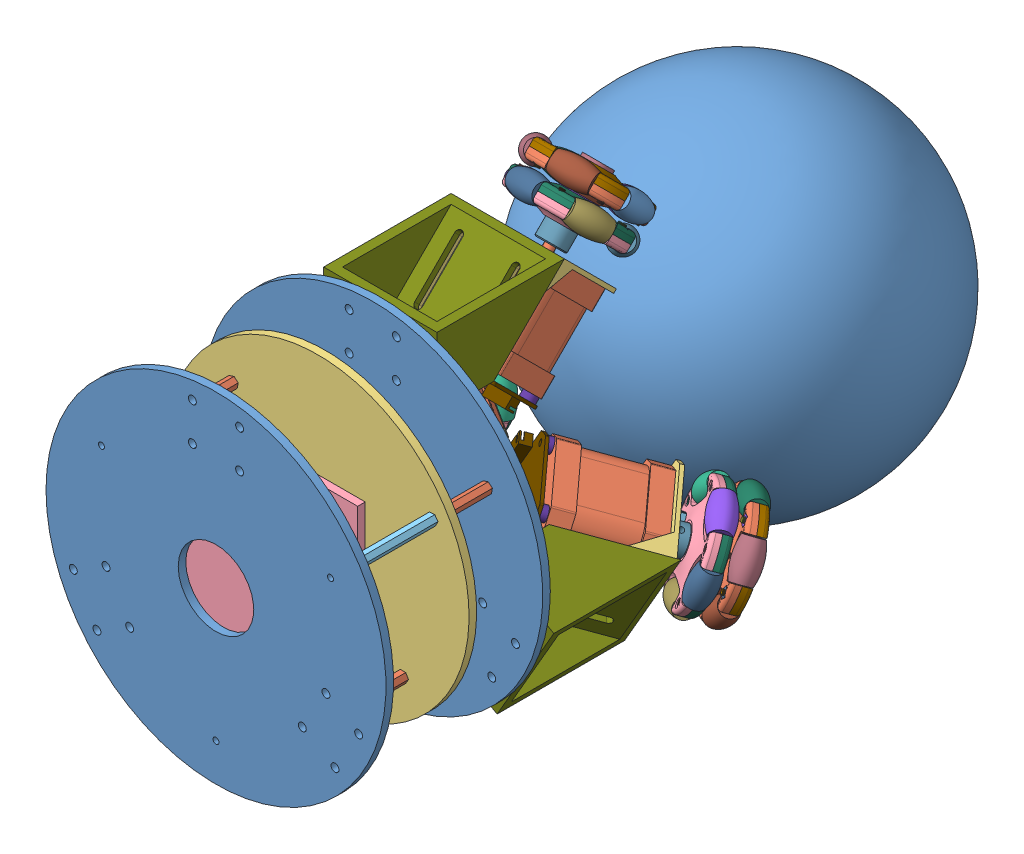
SolidWorks assembly 轮球平衡机器人, configuration 默认. Lengths in mm.
Overall size (282.14 310.32 417.32).
195 component instances, 61 part files, 35 mates.
Components (placement in the parent):
- 底盘底层-1: 底盘底层 [默认] at (0 81.589 0) size (180 180 4)
- 轮电机装配-1: 轮电机装配 [默认] at (-247.6697 -4.8466 -119.7715) x (0.62563 0.330076 -0.70685) z (-0.483308 0.875243 -0.019064) size (112.27 117.96 63.25)
  - 42步进电机-1: 42步进电机 [Default] at (113.7797 -206.2562 -45.9286) x (-0.026961 0 0.999636) z (0 1 0) size (42 47 67.8)
  - 42步进电机连接件-1: 42步进电机连接件 [默认] at (113.7797 -156.4562 -45.9286) x (0.026961 0 -0.999636) z (-0.999636 0 -0.026961) size (50 53 51)
  - 58mm全向轮-2: 58mm全向轮 [默认] at (113.7797 -145.9562 -45.9286) size (67.49 41.74 62.32)
    - 58MMQUANXIANGLUN_DAN-1: 58MMQUANXIANGLUN_DAN [默认] at origin size (67.49 27.49 60.7)
      - DANGPIAN-1-1: DANGPIAN-1 [默认] at origin size (55.41 8.9 53.54)
      - GUNZHOU-1-1: GUNZHOU-1 [默认] at origin size (10.16 3.8 24.74)
      - GUNZI-1-1: GUNZI-1 [默认] at origin size (19.85 20.87 20.84)
      - GUNZHOU_1-1-1: GUNZHOU_1-1 [默认] at origin size (25.2 3.8 3.8)
      - GUNZI_1-1-1: GUNZI_1-1 [默认] at origin size (19.2 13.87 13.87)
      - GUNZHOU_2-1-1: GUNZHOU_2-1 [默认] at origin size (10.16 3.8 24.74)
      - GUNZI_2-1-1: GUNZI_2-1 [默认] at origin size (19.85 20.87 20.84)
      - GUNZHOU_3-1-1: GUNZHOU_3-1 [默认] at origin size (21.86 3.8 16.83)
      - GUNZI_3-1-1: GUNZI_3-1 [默认] at origin size (20.83 27.49 22.24)
      - GUNZHOU_4-1-1: GUNZHOU_4-1 [默认] at origin size (21.86 3.8 16.83)
      - GUNZI_4-1-1: GUNZI_4-1 [默认] at origin size (20.83 27.49 22.24)
      - DANGPIAN_HOU-1-1: DANGPIAN_HOU-1 [默认] at origin size (55.39 8.9 53.54)
      - M3X8-1-1: M3X8-1 [默认] at origin size (4.21 9.65 4.2)
      - M3LUOMU-1-1: M3LUOMU-1 [默认] at origin size (4.9 2 5.66)
      - M3X8_1-1-1: M3X8_1-1 [默认] at origin size (4.2 9.65 4.2)
      - M3LUOMU_1-1-1: M3LUOMU_1-1 [默认] at origin size (5.38 2 5.53)
      - M3X8_2-1-1: M3X8_2-1 [默认] at origin size (4.2 9.65 4.2)
      - M3LUOMU_2-1-1: M3LUOMU_2-1 [默认] at origin size (5.63 2 5.17)
      - M3X8_3-1-1: M3X8_3-1 [默认] at origin size (4.2 9.65 4.2)
      - M3LUOMU_3-1-1: M3LUOMU_3-1 [默认] at origin size (5.63 2 5.17)
      - M3X8_4-1-1: M3X8_4-1 [默认] at origin size (4.2 9.65 4.2)
      - M3LUOMU_4-1-1: M3LUOMU_4-1 [默认] at origin size (5.38 2 5.53)
    - LIANJIEQUAN-1-1: LIANJIEQUAN-1 [默认] at origin size (17 2.5 17)
    - 58MMQUANXIANGLUN_DAN_1-1: 58MMQUANXIANGLUN_DAN_1 [默认] at origin size (67.49 27.49 60.7)
      - DANGPIAN-3-1: DANGPIAN-3 [默认] at origin size (55.41 8.9 53.54)
      - GUNZHOU-3-1: GUNZHOU-3 [默认] at origin size (10.16 3.8 24.74)
      - GUNZI-3-1: GUNZI-3 [默认] at origin size (19.85 20.87 20.84)
      - GUNZHOU_1-3-1: GUNZHOU_1-3 [默认] at origin size (21.86 3.8 16.83)
      - GUNZI_1-3-1: GUNZI_1-3 [默认] at origin size (20.83 27.49 22.24)
      - GUNZHOU_2-3-1: GUNZHOU_2-3 [默认] at origin size (21.86 3.8 16.83)
      - GUNZI_2-3-1: GUNZI_2-3 [默认] at origin size (20.83 27.49 22.24)
      - GUNZHOU_3-3-1: GUNZHOU_3-3 [默认] at origin size (10.16 3.8 24.74)
      - GUNZI_3-3-1: GUNZI_3-3 [默认] at origin size (19.85 20.87 20.84)
      - GUNZHOU_4-3-1: GUNZHOU_4-3 [默认] at origin size (25.2 3.8 3.8)
      - GUNZI_4-3-1: GUNZI_4-3 [默认] at origin size (19.2 13.87 13.87)
      - DANGPIAN_HOU-3-1: DANGPIAN_HOU-3 [默认] at origin size (55.39 8.9 53.54)
      - M3X8-3-1: M3X8-3 [默认] at origin size (4.2 9.65 4.2)
      - M3LUOMU-3-1: M3LUOMU-3 [默认] at origin size (5.63 2 5.17)
      - M3X8_1-3-1: M3X8_1-3 [默认] at origin size (4.2 9.65 4.2)
      - M3LUOMU_1-3-1: M3LUOMU_1-3 [默认] at origin size (5.38 2 5.53)
      - M3X8_2-3-1: M3X8_2-3 [默认] at origin size (4.21 9.65 4.2)
      - M3LUOMU_2-3-1: M3LUOMU_2-3 [默认] at origin size (4.9 2 5.66)
      - M3X8_3-3-1: M3X8_3-3 [默认] at origin size (4.2 9.65 4.2)
      - M3LUOMU_3-3-1: M3LUOMU_3-3 [默认] at origin size (5.38 2 5.53)
      - M3X8_4-3-1: M3X8_4-3 [默认] at origin size (4.2 9.65 4.2)
      - M3LUOMU_4-3-1: M3LUOMU_4-3 [默认] at origin size (5.63 2 5.17)
    - 20170615_LIANZHOUQITAOJIAN4X23-1-1: 20170615_LIANZHOUQITAOJIAN4X23-1 [默认] at origin size (13.9 6 13.9)
    - 20170615_LIANZHOUQI_4X23-1-1: 20170615_LIANZHOUQI_4X23-1 [默认] at origin size (13.9 23 13.9)
    - M4X12-1-1: M4X12-1 [默认] at origin size (6.9 15.15 7.04)
  - 底盘连接件-1: 底盘连接件 [默认] at (84.5995 -209.4562 -76.7265) x (-0.026961 0 0.999636) z (0.70685 -0.707107 0.019064) size (60 67.48 37.48)
  - 3mm尼龙垫圈高度3mm-1: 3mm尼龙垫圈高度3mm [默认] at (129.692 -209.2562 -61.0051) size (7 3 7)
  - 3mm尼龙垫圈高度3mm-2: 3mm尼龙垫圈高度3mm [默认] at (128.8562 -209.2562 -30.0163) size (7 3 7)
  - 3mm尼龙垫圈高度3mm-3: 3mm尼龙垫圈高度3mm [默认] at (98.7033 -209.2562 -61.8408) size (7 3 7)
  - 3mm尼龙垫圈高度3mm-4: 3mm尼龙垫圈高度3mm [默认] at (97.8675 -209.2562 -30.8521) size (7 3 7)
  - 42闭环PCB-1: 42闭环PCB [默认] at (98.7033 -209.2562 -61.8408) x (-1 0 0) z (0 -1 0) size (46.56 42.8 7)
- 轮电机装配-4: 轮电机装配 [默认] at (48.9795 339.2949 -119.7715) x (-0.026961 -0.70685 -0.70685) z (0.999636 -0.019064 -0.019064) size (112.27 117.96 63.25)
  - 42步进电机-1: 42步进电机 [Default] at (113.7797 -206.2562 -45.9286) x (-0.026961 0 0.999636) z (0 1 0) size (42 47 67.8)
  - 42步进电机连接件-1: 42步进电机连接件 [默认] at (113.7797 -156.4562 -45.9286) x (0.026961 0 -0.999636) z (-0.999636 0 -0.026961) size (50 53 51)
  - 58mm全向轮-2: 58mm全向轮 [默认] at (113.7797 -145.9562 -45.9286) size (67.49 41.74 62.32)
    - 58MMQUANXIANGLUN_DAN-1: 58MMQUANXIANGLUN_DAN [默认] at origin size (67.49 27.49 60.7)
      - DANGPIAN-1-1: DANGPIAN-1 [默认] at origin size (55.41 8.9 53.54)
      - GUNZHOU-1-1: GUNZHOU-1 [默认] at origin size (10.16 3.8 24.74)
      - GUNZI-1-1: GUNZI-1 [默认] at origin size (19.85 20.87 20.84)
      - GUNZHOU_1-1-1: GUNZHOU_1-1 [默认] at origin size (25.2 3.8 3.8)
      - GUNZI_1-1-1: GUNZI_1-1 [默认] at origin size (19.2 13.87 13.87)
      - GUNZHOU_2-1-1: GUNZHOU_2-1 [默认] at origin size (10.16 3.8 24.74)
      - GUNZI_2-1-1: GUNZI_2-1 [默认] at origin size (19.85 20.87 20.84)
      - GUNZHOU_3-1-1: GUNZHOU_3-1 [默认] at origin size (21.86 3.8 16.83)
      - GUNZI_3-1-1: GUNZI_3-1 [默认] at origin size (20.83 27.49 22.24)
      - GUNZHOU_4-1-1: GUNZHOU_4-1 [默认] at origin size (21.86 3.8 16.83)
      - GUNZI_4-1-1: GUNZI_4-1 [默认] at origin size (20.83 27.49 22.24)
      - DANGPIAN_HOU-1-1: DANGPIAN_HOU-1 [默认] at origin size (55.39 8.9 53.54)
      - M3X8-1-1: M3X8-1 [默认] at origin size (4.21 9.65 4.2)
      - M3LUOMU-1-1: M3LUOMU-1 [默认] at origin size (4.9 2 5.66)
      - M3X8_1-1-1: M3X8_1-1 [默认] at origin size (4.2 9.65 4.2)
      - M3LUOMU_1-1-1: M3LUOMU_1-1 [默认] at origin size (5.38 2 5.53)
      - M3X8_2-1-1: M3X8_2-1 [默认] at origin size (4.2 9.65 4.2)
      - M3LUOMU_2-1-1: M3LUOMU_2-1 [默认] at origin size (5.63 2 5.17)
      - M3X8_3-1-1: M3X8_3-1 [默认] at origin size (4.2 9.65 4.2)
      - M3LUOMU_3-1-1: M3LUOMU_3-1 [默认] at origin size (5.63 2 5.17)
      - M3X8_4-1-1: M3X8_4-1 [默认] at origin size (4.2 9.65 4.2)
      - M3LUOMU_4-1-1: M3LUOMU_4-1 [默认] at origin size (5.38 2 5.53)
    - LIANJIEQUAN-1-1: LIANJIEQUAN-1 [默认] at origin size (17 2.5 17)
    - 58MMQUANXIANGLUN_DAN_1-1: 58MMQUANXIANGLUN_DAN_1 [默认] at origin size (67.49 27.49 60.7)
      - DANGPIAN-3-1: DANGPIAN-3 [默认] at origin size (55.41 8.9 53.54)
      - GUNZHOU-3-1: GUNZHOU-3 [默认] at origin size (10.16 3.8 24.74)
      - GUNZI-3-1: GUNZI-3 [默认] at origin size (19.85 20.87 20.84)
      - GUNZHOU_1-3-1: GUNZHOU_1-3 [默认] at origin size (21.86 3.8 16.83)
      - GUNZI_1-3-1: GUNZI_1-3 [默认] at origin size (20.83 27.49 22.24)
      - GUNZHOU_2-3-1: GUNZHOU_2-3 [默认] at origin size (21.86 3.8 16.83)
      - GUNZI_2-3-1: GUNZI_2-3 [默认] at origin size (20.83 27.49 22.24)
      - GUNZHOU_3-3-1: GUNZHOU_3-3 [默认] at origin size (10.16 3.8 24.74)
      - GUNZI_3-3-1: GUNZI_3-3 [默认] at origin size (19.85 20.87 20.84)
      - GUNZHOU_4-3-1: GUNZHOU_4-3 [默认] at origin size (25.2 3.8 3.8)
      - GUNZI_4-3-1: GUNZI_4-3 [默认] at origin size (19.2 13.87 13.87)
      - DANGPIAN_HOU-3-1: DANGPIAN_HOU-3 [默认] at origin size (55.39 8.9 53.54)
      - M3X8-3-1: M3X8-3 [默认] at origin size (4.2 9.65 4.2)
      - M3LUOMU-3-1: M3LUOMU-3 [默认] at origin size (5.63 2 5.17)
      - M3X8_1-3-1: M3X8_1-3 [默认] at origin size (4.2 9.65 4.2)
      - M3LUOMU_1-3-1: M3LUOMU_1-3 [默认] at origin size (5.38 2 5.53)
      - M3X8_2-3-1: M3X8_2-3 [默认] at origin size (4.21 9.65 4.2)
      - M3LUOMU_2-3-1: M3LUOMU_2-3 [默认] at origin size (4.9 2 5.66)
      - M3X8_3-3-1: M3X8_3-3 [默认] at origin size (4.2 9.65 4.2)
      - M3LUOMU_3-3-1: M3LUOMU_3-3 [默认] at origin size (5.38 2 5.53)
      - M3X8_4-3-1: M3X8_4-3 [默认] at origin size (4.2 9.65 4.2)
      - M3LUOMU_4-3-1: M3LUOMU_4-3 [默认] at origin size (5.63 2 5.17)
    - 20170615_LIANZHOUQITAOJIAN4X23-1-1: 20170615_LIANZHOUQITAOJIAN4X23-1 [默认] at origin size (13.9 6 13.9)
    - 20170615_LIANZHOUQI_4X23-1-1: 20170615_LIANZHOUQI_4X23-1 [默认] at origin size (13.9 23 13.9)
    - M4X12-1-1: M4X12-1 [默认] at origin size (6.9 15.15 7.04)
  - 底盘连接件-1: 底盘连接件 [默认] at (84.5995 -209.4562 -76.7265) x (-0.026961 0 0.999636) z (0.70685 -0.707107 0.019064) size (60 67.48 37.48)
  - 3mm尼龙垫圈高度3mm-1: 3mm尼龙垫圈高度3mm [默认] at (129.692 -209.2562 -61.0051) size (7 3 7)
  - 3mm尼龙垫圈高度3mm-2: 3mm尼龙垫圈高度3mm [默认] at (128.8562 -209.2562 -30.0163) size (7 3 7)
  - 3mm尼龙垫圈高度3mm-3: 3mm尼龙垫圈高度3mm [默认] at (98.7033 -209.2562 -61.8408) size (7 3 7)
  - 3mm尼龙垫圈高度3mm-4: 3mm尼龙垫圈高度3mm [默认] at (97.8675 -209.2562 -30.8521) size (7 3 7)
  - 42闭环PCB-1: 42闭环PCB [默认] at (98.7033 -209.2562 -61.8408) x (-1 0 0) z (0 -1 0) size (46.56 42.8 7)
- 轮电机装配-5: 轮电机装配 [默认] at (198.6902 -89.6815 -119.7715) x (-0.598669 0.376774 -0.70685) z (-0.516328 -0.856179 -0.019064) size (112.27 117.96 63.25)
  - 42步进电机-1: 42步进电机 [Default] at (113.7797 -206.2562 -45.9286) x (-0.026961 0 0.999636) z (0 1 0) size (42 47 67.8)
  - 42步进电机连接件-1: 42步进电机连接件 [默认] at (113.7797 -156.4562 -45.9286) x (0.026961 0 -0.999636) z (-0.999636 0 -0.026961) size (50 53 51)
  - 58mm全向轮-2: 58mm全向轮 [默认] at (113.7797 -145.9562 -45.9286) size (67.49 41.74 62.32)
    - 58MMQUANXIANGLUN_DAN-1: 58MMQUANXIANGLUN_DAN [默认] at origin size (67.49 27.49 60.7)
      - DANGPIAN-1-1: DANGPIAN-1 [默认] at origin size (55.41 8.9 53.54)
      - GUNZHOU-1-1: GUNZHOU-1 [默认] at origin size (10.16 3.8 24.74)
      - GUNZI-1-1: GUNZI-1 [默认] at origin size (19.85 20.87 20.84)
      - GUNZHOU_1-1-1: GUNZHOU_1-1 [默认] at origin size (25.2 3.8 3.8)
      - GUNZI_1-1-1: GUNZI_1-1 [默认] at origin size (19.2 13.87 13.87)
      - GUNZHOU_2-1-1: GUNZHOU_2-1 [默认] at origin size (10.16 3.8 24.74)
      - GUNZI_2-1-1: GUNZI_2-1 [默认] at origin size (19.85 20.87 20.84)
      - GUNZHOU_3-1-1: GUNZHOU_3-1 [默认] at origin size (21.86 3.8 16.83)
      - GUNZI_3-1-1: GUNZI_3-1 [默认] at origin size (20.83 27.49 22.24)
      - GUNZHOU_4-1-1: GUNZHOU_4-1 [默认] at origin size (21.86 3.8 16.83)
      - GUNZI_4-1-1: GUNZI_4-1 [默认] at origin size (20.83 27.49 22.24)
      - DANGPIAN_HOU-1-1: DANGPIAN_HOU-1 [默认] at origin size (55.39 8.9 53.54)
      - M3X8-1-1: M3X8-1 [默认] at origin size (4.21 9.65 4.2)
      - M3LUOMU-1-1: M3LUOMU-1 [默认] at origin size (4.9 2 5.66)
      - M3X8_1-1-1: M3X8_1-1 [默认] at origin size (4.2 9.65 4.2)
      - M3LUOMU_1-1-1: M3LUOMU_1-1 [默认] at origin size (5.38 2 5.53)
      - M3X8_2-1-1: M3X8_2-1 [默认] at origin size (4.2 9.65 4.2)
      - M3LUOMU_2-1-1: M3LUOMU_2-1 [默认] at origin size (5.63 2 5.17)
      - M3X8_3-1-1: M3X8_3-1 [默认] at origin size (4.2 9.65 4.2)
      - M3LUOMU_3-1-1: M3LUOMU_3-1 [默认] at origin size (5.63 2 5.17)
      - M3X8_4-1-1: M3X8_4-1 [默认] at origin size (4.2 9.65 4.2)
      - M3LUOMU_4-1-1: M3LUOMU_4-1 [默认] at origin size (5.38 2 5.53)
    - LIANJIEQUAN-1-1: LIANJIEQUAN-1 [默认] at origin size (17 2.5 17)
    - 58MMQUANXIANGLUN_DAN_1-1: 58MMQUANXIANGLUN_DAN_1 [默认] at origin size (67.49 27.49 60.7)
      - DANGPIAN-3-1: DANGPIAN-3 [默认] at origin size (55.41 8.9 53.54)
      - GUNZHOU-3-1: GUNZHOU-3 [默认] at origin size (10.16 3.8 24.74)
      - GUNZI-3-1: GUNZI-3 [默认] at origin size (19.85 20.87 20.84)
      - GUNZHOU_1-3-1: GUNZHOU_1-3 [默认] at origin size (21.86 3.8 16.83)
      - GUNZI_1-3-1: GUNZI_1-3 [默认] at origin size (20.83 27.49 22.24)
      - GUNZHOU_2-3-1: GUNZHOU_2-3 [默认] at origin size (21.86 3.8 16.83)
      - GUNZI_2-3-1: GUNZI_2-3 [默认] at origin size (20.83 27.49 22.24)
      - GUNZHOU_3-3-1: GUNZHOU_3-3 [默认] at origin size (10.16 3.8 24.74)
      - GUNZI_3-3-1: GUNZI_3-3 [默认] at origin size (19.85 20.87 20.84)
      - GUNZHOU_4-3-1: GUNZHOU_4-3 [默认] at origin size (25.2 3.8 3.8)
      - GUNZI_4-3-1: GUNZI_4-3 [默认] at origin size (19.2 13.87 13.87)
      - DANGPIAN_HOU-3-1: DANGPIAN_HOU-3 [默认] at origin size (55.39 8.9 53.54)
      - M3X8-3-1: M3X8-3 [默认] at origin size (4.2 9.65 4.2)
      - M3LUOMU-3-1: M3LUOMU-3 [默认] at origin size (5.63 2 5.17)
      - M3X8_1-3-1: M3X8_1-3 [默认] at origin size (4.2 9.65 4.2)
      - M3LUOMU_1-3-1: M3LUOMU_1-3 [默认] at origin size (5.38 2 5.53)
      - M3X8_2-3-1: M3X8_2-3 [默认] at origin size (4.21 9.65 4.2)
      - M3LUOMU_2-3-1: M3LUOMU_2-3 [默认] at origin size (4.9 2 5.66)
      - M3X8_3-3-1: M3X8_3-3 [默认] at origin size (4.2 9.65 4.2)
      - M3LUOMU_3-3-1: M3LUOMU_3-3 [默认] at origin size (5.38 2 5.53)
      - M3X8_4-3-1: M3X8_4-3 [默认] at origin size (4.2 9.65 4.2)
      - M3LUOMU_4-3-1: M3LUOMU_4-3 [默认] at origin size (5.63 2 5.17)
    - 20170615_LIANZHOUQITAOJIAN4X23-1-1: 20170615_LIANZHOUQITAOJIAN4X23-1 [默认] at origin size (13.9 6 13.9)
    - 20170615_LIANZHOUQI_4X23-1-1: 20170615_LIANZHOUQI_4X23-1 [默认] at origin size (13.9 23 13.9)
    - M4X12-1-1: M4X12-1 [默认] at origin size (6.9 15.15 7.04)
  - 底盘连接件-1: 底盘连接件 [默认] at (84.5995 -209.4562 -76.7265) x (-0.026961 0 0.999636) z (0.70685 -0.707107 0.019064) size (60 67.48 37.48)
  - 3mm尼龙垫圈高度3mm-1: 3mm尼龙垫圈高度3mm [默认] at (129.692 -209.2562 -61.0051) size (7 3 7)
  - 3mm尼龙垫圈高度3mm-2: 3mm尼龙垫圈高度3mm [默认] at (128.8562 -209.2562 -30.0163) size (7 3 7)
  - 3mm尼龙垫圈高度3mm-3: 3mm尼龙垫圈高度3mm [默认] at (98.7033 -209.2562 -61.8408) size (7 3 7)
  - 3mm尼龙垫圈高度3mm-4: 3mm尼龙垫圈高度3mm [默认] at (97.8675 -209.2562 -30.8521) size (7 3 7)
  - 42闭环PCB-1: 42闭环PCB [默认] at (98.7033 -209.2562 -61.8408) x (-1 0 0) z (0 -1 0) size (46.56 42.8 7)
- 直径60球体-1: 直径60球体 [默认] at (0.025 81.6034 -189.1818) x (0.722247 0.614016 0.318345) z (0.03945 -0.496101 0.867368) size (180 180 180)
- 铜柱_25MM-1: 铜柱_25MM [默认] at (0 11.589 29) x (0.807015 -0.59053 0) z (0 0 -1) size (5.75 5.22 30.08)
- 铜柱_25MM-3: 铜柱_25MM [默认] at (-60.6218 116.589 29) x (-0.914922 -0.403631 0) z (0 0 -1) size (5.75 5.22 30.08)
- 铜柱_25MM-4: 铜柱_25MM [默认] at (60.6218 116.589 29) x (0.107907 0.994161 0) z (0 0 -1) size (5.75 5.22 30.08)
- 二层连接板-1: 二层连接板 [默认] at (0 81.589 29) x (0.558023 -0.829826 0) z (-0.829826 -0.558023 0) size (160 4 160)
- 电控板-1: 电控板 [默认] at (0.025 81.6034 58) x (0 -1 0) z (0 0 1) size (100 100 4)
- 铜柱_25MM-5: 铜柱_25MM [默认] at (-44.975 126.6034 58) x (0.807015 -0.59053 0) z (0 0 -1) size (5.75 5.22 30.08)
- 铜柱_25MM-6: 铜柱_25MM [默认] at (45.025 36.6034 58) x (0.568708 -0.822539 0) z (0 0 -1) size (5.75 5.22 30.08)
- 铜柱_80MM-1: 铜柱_80MM [默认] at (-60.6218 116.589 33) x (-0.082222 0.996614 0) z (0 0 1) size (5.75 5.22 50)
- 铜柱_80MM-2: 铜柱_80MM [默认] at (60.6218 116.589 33) size (5.75 5.22 50)
- 铜柱_80MM-3: 铜柱_80MM [默认] at (0 11.589 33) size (5.75 5.22 50)
- 配重固定层-1: 配重固定层 [默认] at (0 81.589 87) x (-0.439639 0.898175 0) z (-0.898175 -0.439639 0) size (155 4 155) (hidden)
- 配重块SLDPRT-1: 配重块SLDPRT [默认] at (0.025 127.6034 107) x (1 0 0) z (0 1 0) size (49 20 124) (hidden)
- 底盘底层-2: 底盘底层 [默认] at (0 81.589 83) size (180 180 4)
Mates (geometry in assembly coordinates):
- 重合1: coincident aligned: plane of 底盘底层-1 through (0 81.589 0) normal (0 0 1); plane of assembly through (0 0 0) normal (0 0 1)
- 重合2: coincident aligned: plane of 底盘底层-1 through (0 81.589 0) normal (1 0 0); plane of assembly through (0 0 0) normal (1 0 0)
- 重合3: coincident anti-aligned: plane of 底盘底层-1 through (0 81.589 0) normal (0 0 -1); plane of 轮电机装配-1/底盘连接件-1 through (-31.8939 34.3075 0) normal (0 0 1)
- 同心3: concentric anti-aligned: cylinder of 底盘底层-1 through (-63.032 30.7636 4) axis (0 0 -1) radius 2.1; cylinder of 轮电机装配-1/底盘连接件-1 through (-63.032 30.7636 -5) axis (0 0 1) radius 2.1
- 同心4: concentric anti-aligned: cylinder of 底盘底层-1 through (-58.2115 62.4143 4) axis (0 0 -1) radius 2.1; cylinder of 轮电机装配-1/底盘连接件-1 through (-58.2115 62.4143 -5) axis (0 0 1) radius 2.1
- 重合4: coincident anti-aligned: plane of 底盘底层-1 through (0 81.589 4) normal (0 0 1); plane of 铜柱_25MM-1 through (0 11.589 4) normal (0 0 -1)
- 重合8: coincident anti-aligned: plane of 铜柱_25MM-1 through (0 11.589 29) normal (0 0 1); plane of 二层连接板-1 through (0 81.589 29) normal (0 0 -1)
- 同心5: concentric anti-aligned: cylinder of 铜柱_25MM-3 through (-60.6218 116.589 29) axis (0 0 1) radius 1.25; cylinder of 二层连接板-1 through (-60.6218 116.589 33) axis (0 0 -1) radius 1.6
- 同心6: concentric aligned: cylinder of 底盘底层-1 through (0 81.589 4) axis (0 0 -1) radius 90; cylinder of 二层连接板-1 through (0 81.589 33) axis (0 0 -1) radius 80
- 同心7: concentric anti-aligned: circle of 底盘底层-1; cylinder of 二层连接板-1 through (0 11.589 33) axis (0 0 -1) radius 1.6
- 相切5: tangent: face of 轮电机装配-5/58mm全向轮-2/58MMQUANXIANGLUN_DAN_1-1/GUNZI_3-3-1; sphere of 直径60球体-1
- 相切6: tangent: face of 轮电机装配-4/58mm全向轮-2/58MMQUANXIANGLUN_DAN_1-1/GUNZI_3-3-1; sphere of 直径60球体-1
- 相切7: tangent: face of 轮电机装配-1/58mm全向轮-2/58MMQUANXIANGLUN_DAN-1/GUNZI-1-1; sphere of 直径60球体-1
- 同心8: concentric aligned: circle of 二层连接板-1; circle of 电控板-1
- 同心9: concentric aligned: circle of 二层连接板-1; circle of 电控板-1
- 同心10: concentric aligned: circle of 电控板-1; cylinder of 铜柱_25MM-6 through (45.025 36.6034 58) axis (0 0 1) radius 1.25
- 同心11: concentric anti-aligned: cylinder of 电控板-1 through (-44.975 126.6034 62) axis (0 0 -1) radius 1.5; cylinder of 铜柱_25MM-5 through (-44.975 126.6034 58) axis (0 0 1) radius 1.25
- 重合9: coincident anti-aligned: plane of 电控板-1 through (0.025 81.6034 58) normal (0 0 -1); plane of 铜柱_25MM-5 through (-44.975 126.6034 58) normal (0 0 1)
- 重合10: coincident anti-aligned: plane of 电控板-1 through (0.025 81.6034 58) normal (0 0 -1); plane of 铜柱_25MM-6 through (45.025 36.6034 58) normal (0 0 1)
- 重合11: coincident anti-aligned: plane of 二层连接板-1 through (0 81.589 33) normal (0 0 1); plane of 铜柱_25MM-5 through (-44.975 126.6034 33) normal (0 0 -1)
- 同心13: concentric aligned: circle of 二层连接板-1; circle of 铜柱_80MM-1
- 重合12: coincident anti-aligned: plane of 二层连接板-1 through (0 81.589 33) normal (0 0 1); plane of 铜柱_80MM-1 through (-60.6218 116.589 33) normal (0 0 -1)
- 同心14: concentric aligned: circle of 二层连接板-1; circle of 铜柱_80MM-3
- 同心15: concentric anti-aligned: cylinder of 二层连接板-1 through (60.6218 116.589 33) axis (0 0 -1) radius 1.6; circle of 铜柱_80MM-2
- 重合13: coincident anti-aligned: plane of 二层连接板-1 through (0 81.589 33) normal (0 0 1); plane of 铜柱_80MM-2 through (60.6218 116.589 33) normal (0 0 -1)
- 重合14: coincident anti-aligned: plane of 二层连接板-1 through (0 81.589 33) normal (0 0 1); plane of 铜柱_80MM-3 through (0 11.589 33) normal (0 0 -1)
- 同心16: concentric anti-aligned: circle of 铜柱_80MM-3; circle of 配重固定层-1
- 同心17: concentric anti-aligned: circle of 铜柱_80MM-1; circle of 配重固定层-1
- 重合15: coincident anti-aligned: plane of 铜柱_80MM-3 through (0 11.589 83) normal (0 0 1); plane of 配重固定层-1 through (0 81.589 83) normal (0 0 -1)
- 重合16: coincident anti-aligned: plane of 配重固定层-1 through (0 81.589 87) normal (0 0 1); plane of 配重块SLDPRT-1 through (0.025 127.6034 87) normal (0 0 -1)
- 重合17: coincident aligned: plane of 电控板-1; plane of 配重块SLDPRT-1
- 重合18: coincident aligned: plane of 电控板-1; plane of 配重块SLDPRT-1
- 同心18: concentric anti-aligned: cylinder of 铜柱_80MM-2 through (60.6218 116.589 33) axis (0 0 -1) radius 1.25; cylinder of 底盘底层-2 through (60.6218 116.589 77) axis (0 0 1) radius 1.6
- 同心19: concentric anti-aligned: cylinder of 铜柱_80MM-1 through (-60.6218 116.589 33) axis (0 0 -1) radius 1.25; cylinder of 底盘底层-2 through (-60.6218 116.589 77) axis (0 0 1) radius 1.6
- 重合19: coincident anti-aligned: plane of 铜柱_80MM-3 through (0 11.589 83) normal (0 0 1); plane of 底盘底层-2 through (0 81.589 83) normal (0 0 -1)
